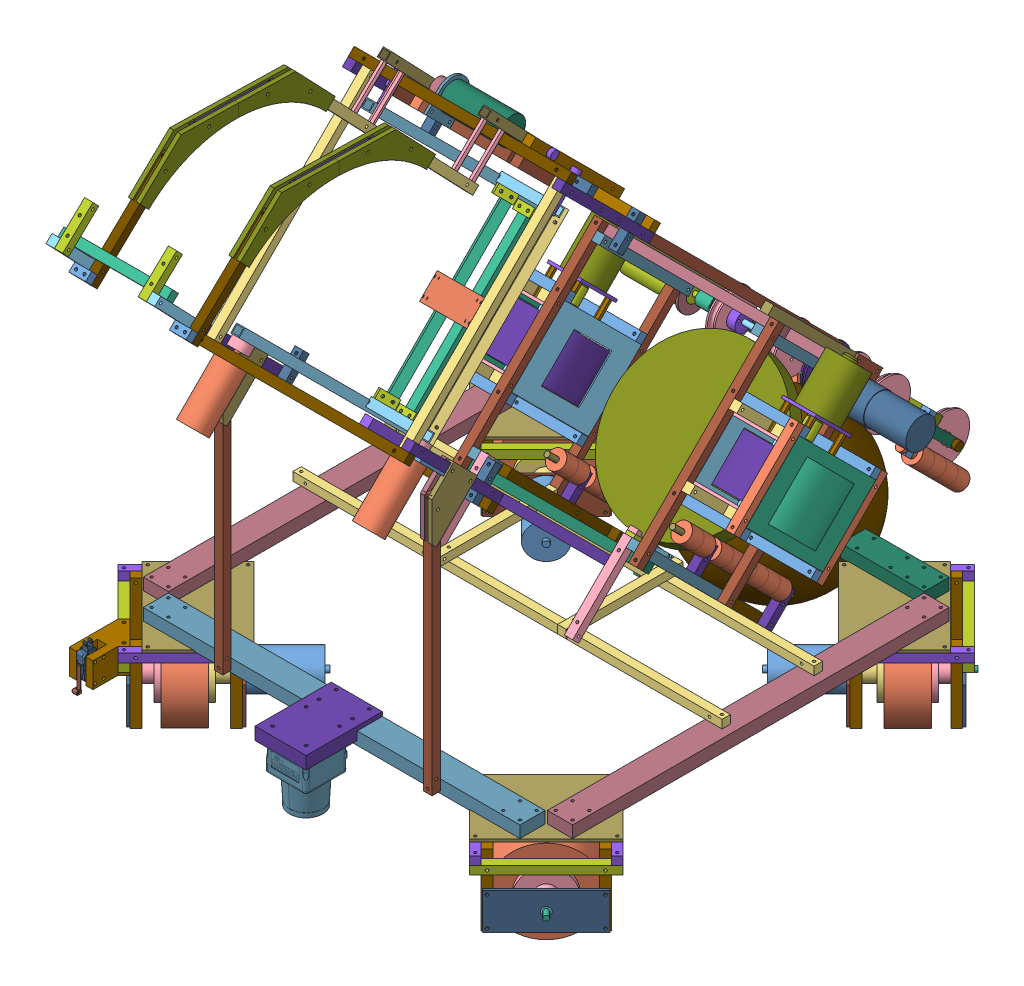
SolidWorks assembly R2, configuration ﾃﾞﾌｫﾙﾄ. Lengths in mm.
Overall size (675.42 1062.97 1046.24).
340 component instances, 123 part files, 65 mates.
Components (placement in the parent):
- Copy of Runner^R2-1: Copy of Runner^R2 [ﾃﾞﾌｫﾙﾄ] at (-280.0303 -23.0504 467.0696) size (603.46 149.94 603.46) (virtual)
  - Copy of Copy of 足回り角^Copy of Runner_R2-1: Copy of Copy of 足回り角^Copy of Runner_R2 [ﾃﾞﾌｫﾙﾄ] at (-236.5804 -569.4039 -424.4309) x (0.322664 -0.429464 -0.843474) z (-0.833839 -0.550655 -0.038606) size (175.41 194.61 181.45) (virtual)
    - Copy of 足回りモータ^Copy of Copy of 足回り角_Copy of Runner_R2-1: Copy of 足回りモータ^Copy of Copy of 足回り角_Copy of Runner_R2 [ﾃﾞﾌｫﾙﾄ] at (-551.1259 26.8519 -574.9243) x (0.279393 -0.550081 -0.786989) z (0.886746 0.462184 -0.008244) size (42 98.4 42) (virtual)
    - Copy of 足回りE^Copy of Copy of 足回り角_Copy of Runner_R2-1: Copy of 足回りE^Copy of Copy of 足回り角_Copy of Runner_R2 [ﾃﾞﾌｫﾙﾄ] at (-524.7579 -22.9499 -530.7534) x (0.201013 -0.588283 -0.783273) z (0.907729 0.412462 -0.07683) size (100 40 100) (virtual)
    - Copy of Part11^Copy of Copy of 足回り角_Copy of Runner_R2-1: Copy of Part11^Copy of Copy of 足回り角_Copy of Runner_R2 [ﾃﾞﾌｫﾙﾄ] at (-688.5751 -7.1777 -584.6401) x (-0.368269 0.695555 -0.616912) z (-0.201013 0.588283 0.783273) size (26.4 56.8 56.8) (virtual)
    - Copy of Copy of Part11^Copy of Copy of 足回り角_Copy of Runner_R2-1: Copy of Copy of Part11^Copy of Copy of 足回り角_Copy of Runner_R2 [ﾃﾞﾌｫﾙﾄ] at (-522.8714 -163.2458 -585.4385) x (0.368269 -0.695555 0.616912) z (0.915702 0.156572 -0.370101) size (26.4 56.8 56.8) (virtual)
    - Part4^Copy of Copy of 足回り角_Copy of Runner_R2-7: Part4^Copy of Copy of 足回り角_Copy of Runner_R2 [ﾃﾞﾌｫﾙﾄ] at (-186.4359 394.8707 -734.6433) x (-0.368269 0.695555 -0.616912) z (0.907729 0.412462 -0.07683) size (2 10 10) (virtual)
    - Part5^Copy of Copy of 足回り角_Copy of Runner_R2-1: Part5^Copy of Copy of 足回り角_Copy of Runner_R2 [ﾃﾞﾌｫﾙﾄ] at (-68.1457 171.4539 -536.4872) x (0.907729 0.412462 -0.07683) z (0.368269 -0.695555 0.616912) size (6 6 35) (virtual)
    - Part6^Copy of Copy of 足回り角_Copy of Runner_R2-12: Part6^Copy of Copy of 足回り角_Copy of Runner_R2 [ﾃﾞﾌｫﾙﾄ] at (-467.3947 -89.0148 -566.7968) x (0.824584 -0.062152 -0.562315) z (-0.429464 -0.715779 -0.550655) size (130 10 10) (virtual)
    - Part6^Copy of Copy of 足回り角_Copy of Runner_R2-16: Part6^Copy of Copy of 足回り角_Copy of Runner_R2 [ﾃﾞﾌｫﾙﾄ] at (-520.2575 -4.441 -653.6633) x (0.824584 -0.062152 -0.562315) z (0.429464 0.715779 0.550655) size (130 10 10) (virtual)
    - Copy of Part6^Copy of Copy of 足回り角_Copy of Runner_R2-7: Copy of Part6^Copy of Copy of 足回り角_Copy of Runner_R2 [ﾃﾞﾌｫﾙﾄ] at (-544.6117 -11.2666 -643.957) x (-0.368269 0.695555 -0.616912) z (0.429464 0.715779 0.550655) size (115 10 10) (virtual)
    - Copy of Part6^Copy of Copy of 足回り角_Copy of Runner_R2-9: Copy of Part6^Copy of Copy of 足回り角_Copy of Runner_R2 [ﾃﾞﾌｫﾙﾄ] at (-643.5618 -3.8083 -576.4793) x (-0.368269 0.695555 -0.616912) z (0.429464 0.715779 0.550655) size (115 10 10) (virtual)
    - Copy of Copy of Part6^Copy of Copy of 足回り角_Copy of Runner_R2-1: Copy of Copy of Part6^Copy of Copy of 足回り角_Copy of Runner_R2 [ﾃﾞﾌｫﾙﾄ] at (-546.4038 -4.8062 -484.4742) x (0.429464 0.715779 0.550655) z (-0.824584 0.062152 0.562315) size (85 10 10) (virtual)
    - Copy of Copy of Part6^Copy of Copy of 足回り角_Copy of Runner_R2-2: Copy of Copy of Part6^Copy of Copy of 足回り角_Copy of Runner_R2 [ﾃﾞﾌｫﾙﾄ] at (-577.7066 54.316 -536.9118) x (0.429464 0.715779 0.550655) z (-0.824584 0.062152 0.562315) size (85 10 10) (virtual)
    - Copy of Copy of Part6^Copy of Copy of 足回り角_Copy of Runner_R2-3: Copy of Copy of Part6^Copy of Copy of 足回り角_Copy of Runner_R2 [ﾃﾞﾌｫﾙﾄ] at (-463.9454 -11.0215 -540.7057) x (0.429464 0.715779 0.550655) z (-0.824584 0.062152 0.562315) size (85 10 10) (virtual)
    - Copy of Copy of Part6^Copy of Copy of 足回り角_Copy of Runner_R2-4: Copy of Copy of Part6^Copy of Copy of 足回り角_Copy of Runner_R2 [ﾃﾞﾌｫﾙﾄ] at (-495.2482 48.1008 -593.1432) x (0.429464 0.715779 0.550655) z (-0.824584 0.062152 0.562315) size (85 10 10) (virtual)
    - Copy of Part7^Copy of Copy of 足回り角_Copy of Runner_R2-1: Copy of Part7^Copy of Copy of 足回り角_Copy of Runner_R2 [ﾃﾞﾌｫﾙﾄ] at (-536.2553 -8.1719 -459.5715) x (0.429464 0.715779 0.550655) z (-0.368269 0.695555 -0.616912) size (43 108 3) (virtual)
    - Part7^Copy of Copy of 足回り角_Copy of Runner_R2-3: Part7^Copy of Copy of 足回り角_Copy of Runner_R2 [ﾃﾞﾌｫﾙﾄ] at (-584.534 59.789 -512.9824) x (0.429464 0.715779 0.550655) z (-0.368269 0.695555 -0.616912) size (43 108 3) (virtual)
    - Part10^Copy of Copy of 足回り角_Copy of Runner_R2-2: Part10^Copy of Copy of 足回り角_Copy of Runner_R2 [ﾃﾞﾌｫﾙﾄ] at (-643.5618 -3.8083 -576.4793) x (0.368269 -0.695555 0.616912) z (-0.429464 -0.715779 -0.550655) size (94.7 130 3) (virtual)
  - Copy of Copy of 足回り角^Copy of Runner_R2-2: Copy of Copy of 足回り角^Copy of Runner_R2 [ﾃﾞﾌｫﾙﾄ] at (937.2593 -569.4039 -236.5804) x (0.843474 -0.429464 0.322664) z (0.038606 -0.550655 -0.833839) size (175.41 194.61 181.45) (virtual)
    - Copy of 足回りモータ^Copy of Copy of 足回り角_Copy of Runner_R2-1: Copy of 足回りモータ^Copy of Copy of 足回り角_Copy of Runner_R2 [ﾃﾞﾌｫﾙﾄ] at (-551.1259 26.8519 -574.9243) x (0.279393 -0.550081 -0.786989) z (0.886746 0.462184 -0.008244) size (42 98.4 42) (virtual)
    - Copy of 足回りE^Copy of Copy of 足回り角_Copy of Runner_R2-1: Copy of 足回りE^Copy of Copy of 足回り角_Copy of Runner_R2 [ﾃﾞﾌｫﾙﾄ] at (-524.7579 -22.9499 -530.7534) x (0.201013 -0.588283 -0.783273) z (0.907729 0.412462 -0.07683) size (100 40 100) (virtual)
    - Copy of Part11^Copy of Copy of 足回り角_Copy of Runner_R2-1: Copy of Part11^Copy of Copy of 足回り角_Copy of Runner_R2 [ﾃﾞﾌｫﾙﾄ] at (-688.5751 -7.1777 -584.6401) x (-0.368269 0.695555 -0.616912) z (-0.201013 0.588283 0.783273) size (26.4 56.8 56.8) (virtual)
    - Copy of Copy of Part11^Copy of Copy of 足回り角_Copy of Runner_R2-1: Copy of Copy of Part11^Copy of Copy of 足回り角_Copy of Runner_R2 [ﾃﾞﾌｫﾙﾄ] at (-522.8714 -163.2458 -585.4385) x (0.368269 -0.695555 0.616912) z (0.915702 0.156572 -0.370101) size (26.4 56.8 56.8) (virtual)
    - Part4^Copy of Copy of 足回り角_Copy of Runner_R2-7: Part4^Copy of Copy of 足回り角_Copy of Runner_R2 [ﾃﾞﾌｫﾙﾄ] at (-186.4359 394.8707 -734.6433) x (-0.368269 0.695555 -0.616912) z (0.907729 0.412462 -0.07683) size (2 10 10) (virtual)
    - Part5^Copy of Copy of 足回り角_Copy of Runner_R2-1: Part5^Copy of Copy of 足回り角_Copy of Runner_R2 [ﾃﾞﾌｫﾙﾄ] at (-68.1457 171.4539 -536.4872) x (0.907729 0.412462 -0.07683) z (0.368269 -0.695555 0.616912) size (6 6 35) (virtual)
    - Part6^Copy of Copy of 足回り角_Copy of Runner_R2-12: Part6^Copy of Copy of 足回り角_Copy of Runner_R2 [ﾃﾞﾌｫﾙﾄ] at (-467.3947 -89.0148 -566.7968) x (0.824584 -0.062152 -0.562315) z (-0.429464 -0.715779 -0.550655) size (130 10 10) (virtual)
    - Part6^Copy of Copy of 足回り角_Copy of Runner_R2-16: Part6^Copy of Copy of 足回り角_Copy of Runner_R2 [ﾃﾞﾌｫﾙﾄ] at (-520.2575 -4.441 -653.6633) x (0.824584 -0.062152 -0.562315) z (0.429464 0.715779 0.550655) size (130 10 10) (virtual)
    - Copy of Part6^Copy of Copy of 足回り角_Copy of Runner_R2-7: Copy of Part6^Copy of Copy of 足回り角_Copy of Runner_R2 [ﾃﾞﾌｫﾙﾄ] at (-544.6117 -11.2666 -643.957) x (-0.368269 0.695555 -0.616912) z (0.429464 0.715779 0.550655) size (115 10 10) (virtual)
    - Copy of Part6^Copy of Copy of 足回り角_Copy of Runner_R2-9: Copy of Part6^Copy of Copy of 足回り角_Copy of Runner_R2 [ﾃﾞﾌｫﾙﾄ] at (-643.5618 -3.8083 -576.4793) x (-0.368269 0.695555 -0.616912) z (0.429464 0.715779 0.550655) size (115 10 10) (virtual)
    - Copy of Copy of Part6^Copy of Copy of 足回り角_Copy of Runner_R2-1: Copy of Copy of Part6^Copy of Copy of 足回り角_Copy of Runner_R2 [ﾃﾞﾌｫﾙﾄ] at (-546.4038 -4.8062 -484.4742) x (0.429464 0.715779 0.550655) z (-0.824584 0.062152 0.562315) size (85 10 10) (virtual)
    - Copy of Copy of Part6^Copy of Copy of 足回り角_Copy of Runner_R2-2: Copy of Copy of Part6^Copy of Copy of 足回り角_Copy of Runner_R2 [ﾃﾞﾌｫﾙﾄ] at (-577.7066 54.316 -536.9118) x (0.429464 0.715779 0.550655) z (-0.824584 0.062152 0.562315) size (85 10 10) (virtual)
    - Copy of Copy of Part6^Copy of Copy of 足回り角_Copy of Runner_R2-3: Copy of Copy of Part6^Copy of Copy of 足回り角_Copy of Runner_R2 [ﾃﾞﾌｫﾙﾄ] at (-463.9454 -11.0215 -540.7057) x (0.429464 0.715779 0.550655) z (-0.824584 0.062152 0.562315) size (85 10 10) (virtual)
    - Copy of Copy of Part6^Copy of Copy of 足回り角_Copy of Runner_R2-4: Copy of Copy of Part6^Copy of Copy of 足回り角_Copy of Runner_R2 [ﾃﾞﾌｫﾙﾄ] at (-495.2482 48.1008 -593.1432) x (0.429464 0.715779 0.550655) z (-0.824584 0.062152 0.562315) size (85 10 10) (virtual)
    - Copy of Part7^Copy of Copy of 足回り角_Copy of Runner_R2-1: Copy of Part7^Copy of Copy of 足回り角_Copy of Runner_R2 [ﾃﾞﾌｫﾙﾄ] at (-536.2553 -8.1719 -459.5715) x (0.429464 0.715779 0.550655) z (-0.368269 0.695555 -0.616912) size (43 108 3) (virtual)
    - Part7^Copy of Copy of 足回り角_Copy of Runner_R2-3: Part7^Copy of Copy of 足回り角_Copy of Runner_R2 [ﾃﾞﾌｫﾙﾄ] at (-584.534 59.789 -512.9824) x (0.429464 0.715779 0.550655) z (-0.368269 0.695555 -0.616912) size (43 108 3) (virtual)
    - Part10^Copy of Copy of 足回り角_Copy of Runner_R2-2: Part10^Copy of Copy of 足回り角_Copy of Runner_R2 [ﾃﾞﾌｫﾙﾄ] at (-643.5618 -3.8083 -576.4793) x (0.368269 -0.695555 0.616912) z (-0.429464 -0.715779 -0.550655) size (94.7 130 3) (virtual)
  - Copy of Copy of 足回り角^Copy of Runner_R2-3: Copy of Copy of 足回り角^Copy of Runner_R2 [ﾃﾞﾌｫﾙﾄ] at (-424.4309 -569.4039 749.4088) x (-0.843474 -0.429464 -0.322664) z (-0.038606 -0.550655 0.833839) size (175.41 194.61 181.45) (virtual)
    - Copy of 足回りモータ^Copy of Copy of 足回り角_Copy of Runner_R2-1: Copy of 足回りモータ^Copy of Copy of 足回り角_Copy of Runner_R2 [ﾃﾞﾌｫﾙﾄ] at (-551.1259 26.8519 -574.9243) x (0.279393 -0.550081 -0.786989) z (0.886746 0.462184 -0.008244) size (42 98.4 42) (virtual)
    - Copy of 足回りE^Copy of Copy of 足回り角_Copy of Runner_R2-1: Copy of 足回りE^Copy of Copy of 足回り角_Copy of Runner_R2 [ﾃﾞﾌｫﾙﾄ] at (-524.7579 -22.9499 -530.7534) x (0.201013 -0.588283 -0.783273) z (0.907729 0.412462 -0.07683) size (100 40 100) (virtual)
    - Copy of Part11^Copy of Copy of 足回り角_Copy of Runner_R2-1: Copy of Part11^Copy of Copy of 足回り角_Copy of Runner_R2 [ﾃﾞﾌｫﾙﾄ] at (-688.5751 -7.1777 -584.6401) x (-0.368269 0.695555 -0.616912) z (-0.201013 0.588283 0.783273) size (26.4 56.8 56.8) (virtual)
    - Copy of Copy of Part11^Copy of Copy of 足回り角_Copy of Runner_R2-1: Copy of Copy of Part11^Copy of Copy of 足回り角_Copy of Runner_R2 [ﾃﾞﾌｫﾙﾄ] at (-522.8714 -163.2458 -585.4385) x (0.368269 -0.695555 0.616912) z (0.915702 0.156572 -0.370101) size (26.4 56.8 56.8) (virtual)
    - Part4^Copy of Copy of 足回り角_Copy of Runner_R2-7: Part4^Copy of Copy of 足回り角_Copy of Runner_R2 [ﾃﾞﾌｫﾙﾄ] at (-186.4359 394.8707 -734.6433) x (-0.368269 0.695555 -0.616912) z (0.907729 0.412462 -0.07683) size (2 10 10) (virtual)
    - Part5^Copy of Copy of 足回り角_Copy of Runner_R2-1: Part5^Copy of Copy of 足回り角_Copy of Runner_R2 [ﾃﾞﾌｫﾙﾄ] at (-68.1457 171.4539 -536.4872) x (0.907729 0.412462 -0.07683) z (0.368269 -0.695555 0.616912) size (6 6 35) (virtual)
    - Part6^Copy of Copy of 足回り角_Copy of Runner_R2-12: Part6^Copy of Copy of 足回り角_Copy of Runner_R2 [ﾃﾞﾌｫﾙﾄ] at (-467.3947 -89.0148 -566.7968) x (0.824584 -0.062152 -0.562315) z (-0.429464 -0.715779 -0.550655) size (130 10 10) (virtual)
    - Part6^Copy of Copy of 足回り角_Copy of Runner_R2-16: Part6^Copy of Copy of 足回り角_Copy of Runner_R2 [ﾃﾞﾌｫﾙﾄ] at (-520.2575 -4.441 -653.6633) x (0.824584 -0.062152 -0.562315) z (0.429464 0.715779 0.550655) size (130 10 10) (virtual)
    - Copy of Part6^Copy of Copy of 足回り角_Copy of Runner_R2-7: Copy of Part6^Copy of Copy of 足回り角_Copy of Runner_R2 [ﾃﾞﾌｫﾙﾄ] at (-544.6117 -11.2666 -643.957) x (-0.368269 0.695555 -0.616912) z (0.429464 0.715779 0.550655) size (115 10 10) (virtual)
    - Copy of Part6^Copy of Copy of 足回り角_Copy of Runner_R2-9: Copy of Part6^Copy of Copy of 足回り角_Copy of Runner_R2 [ﾃﾞﾌｫﾙﾄ] at (-643.5618 -3.8083 -576.4793) x (-0.368269 0.695555 -0.616912) z (0.429464 0.715779 0.550655) size (115 10 10) (virtual)
    - Copy of Copy of Part6^Copy of Copy of 足回り角_Copy of Runner_R2-1: Copy of Copy of Part6^Copy of Copy of 足回り角_Copy of Runner_R2 [ﾃﾞﾌｫﾙﾄ] at (-546.4038 -4.8062 -484.4742) x (0.429464 0.715779 0.550655) z (-0.824584 0.062152 0.562315) size (85 10 10) (virtual)
    - Copy of Copy of Part6^Copy of Copy of 足回り角_Copy of Runner_R2-2: Copy of Copy of Part6^Copy of Copy of 足回り角_Copy of Runner_R2 [ﾃﾞﾌｫﾙﾄ] at (-577.7066 54.316 -536.9118) x (0.429464 0.715779 0.550655) z (-0.824584 0.062152 0.562315) size (85 10 10) (virtual)
    - Copy of Copy of Part6^Copy of Copy of 足回り角_Copy of Runner_R2-3: Copy of Copy of Part6^Copy of Copy of 足回り角_Copy of Runner_R2 [ﾃﾞﾌｫﾙﾄ] at (-463.9454 -11.0215 -540.7057) x (0.429464 0.715779 0.550655) z (-0.824584 0.062152 0.562315) size (85 10 10) (virtual)
    - Copy of Copy of Part6^Copy of Copy of 足回り角_Copy of Runner_R2-4: Copy of Copy of Part6^Copy of Copy of 足回り角_Copy of Runner_R2 [ﾃﾞﾌｫﾙﾄ] at (-495.2482 48.1008 -593.1432) x (0.429464 0.715779 0.550655) z (-0.824584 0.062152 0.562315) size (85 10 10) (virtual)
    - Copy of Part7^Copy of Copy of 足回り角_Copy of Runner_R2-1: Copy of Part7^Copy of Copy of 足回り角_Copy of Runner_R2 [ﾃﾞﾌｫﾙﾄ] at (-536.2553 -8.1719 -459.5715) x (0.429464 0.715779 0.550655) z (-0.368269 0.695555 -0.616912) size (43 108 3) (virtual)
    - Part7^Copy of Copy of 足回り角_Copy of Runner_R2-3: Part7^Copy of Copy of 足回り角_Copy of Runner_R2 [ﾃﾞﾌｫﾙﾄ] at (-584.534 59.789 -512.9824) x (0.429464 0.715779 0.550655) z (-0.368269 0.695555 -0.616912) size (43 108 3) (virtual)
    - Part10^Copy of Copy of 足回り角_Copy of Runner_R2-2: Part10^Copy of Copy of 足回り角_Copy of Runner_R2 [ﾃﾞﾌｫﾙﾄ] at (-643.5618 -3.8083 -576.4793) x (0.368269 -0.695555 0.616912) z (-0.429464 -0.715779 -0.550655) size (94.7 130 3) (virtual)
  - Copy of Copy of 足回り角^Copy of Runner_R2-4: Copy of Copy of 足回り角^Copy of Runner_R2 [ﾃﾞﾌｫﾙﾄ] at (749.4088 -569.4039 937.2593) x (-0.322664 -0.429464 0.843474) z (0.833839 -0.550655 0.038606) size (175.41 194.61 181.45) (virtual)
    - Copy of 足回りモータ^Copy of Copy of 足回り角_Copy of Runner_R2-1: Copy of 足回りモータ^Copy of Copy of 足回り角_Copy of Runner_R2 [ﾃﾞﾌｫﾙﾄ] at (-551.1259 26.8519 -574.9243) x (0.279393 -0.550081 -0.786989) z (0.886746 0.462184 -0.008244) size (42 98.4 42) (virtual)
    - Copy of 足回りE^Copy of Copy of 足回り角_Copy of Runner_R2-1: Copy of 足回りE^Copy of Copy of 足回り角_Copy of Runner_R2 [ﾃﾞﾌｫﾙﾄ] at (-524.7579 -22.9499 -530.7534) x (0.201013 -0.588283 -0.783273) z (0.907729 0.412462 -0.07683) size (100 40 100) (virtual)
    - Copy of Part11^Copy of Copy of 足回り角_Copy of Runner_R2-1: Copy of Part11^Copy of Copy of 足回り角_Copy of Runner_R2 [ﾃﾞﾌｫﾙﾄ] at (-688.5751 -7.1777 -584.6401) x (-0.368269 0.695555 -0.616912) z (-0.201013 0.588283 0.783273) size (26.4 56.8 56.8) (virtual)
    - Copy of Copy of Part11^Copy of Copy of 足回り角_Copy of Runner_R2-1: Copy of Copy of Part11^Copy of Copy of 足回り角_Copy of Runner_R2 [ﾃﾞﾌｫﾙﾄ] at (-522.8714 -163.2458 -585.4385) x (0.368269 -0.695555 0.616912) z (0.915702 0.156572 -0.370101) size (26.4 56.8 56.8) (virtual)
    - Part4^Copy of Copy of 足回り角_Copy of Runner_R2-7: Part4^Copy of Copy of 足回り角_Copy of Runner_R2 [ﾃﾞﾌｫﾙﾄ] at (-186.4359 394.8707 -734.6433) x (-0.368269 0.695555 -0.616912) z (0.907729 0.412462 -0.07683) size (2 10 10) (virtual)
    - Part5^Copy of Copy of 足回り角_Copy of Runner_R2-1: Part5^Copy of Copy of 足回り角_Copy of Runner_R2 [ﾃﾞﾌｫﾙﾄ] at (-68.1457 171.4539 -536.4872) x (0.907729 0.412462 -0.07683) z (0.368269 -0.695555 0.616912) size (6 6 35) (virtual)
    - Part6^Copy of Copy of 足回り角_Copy of Runner_R2-12: Part6^Copy of Copy of 足回り角_Copy of Runner_R2 [ﾃﾞﾌｫﾙﾄ] at (-467.3947 -89.0148 -566.7968) x (0.824584 -0.062152 -0.562315) z (-0.429464 -0.715779 -0.550655) size (130 10 10) (virtual)
    - Part6^Copy of Copy of 足回り角_Copy of Runner_R2-16: Part6^Copy of Copy of 足回り角_Copy of Runner_R2 [ﾃﾞﾌｫﾙﾄ] at (-520.2575 -4.441 -653.6633) x (0.824584 -0.062152 -0.562315) z (0.429464 0.715779 0.550655) size (130 10 10) (virtual)
    - Copy of Part6^Copy of Copy of 足回り角_Copy of Runner_R2-7: Copy of Part6^Copy of Copy of 足回り角_Copy of Runner_R2 [ﾃﾞﾌｫﾙﾄ] at (-544.6117 -11.2666 -643.957) x (-0.368269 0.695555 -0.616912) z (0.429464 0.715779 0.550655) size (115 10 10) (virtual)
    - Copy of Part6^Copy of Copy of 足回り角_Copy of Runner_R2-9: Copy of Part6^Copy of Copy of 足回り角_Copy of Runner_R2 [ﾃﾞﾌｫﾙﾄ] at (-643.5618 -3.8083 -576.4793) x (-0.368269 0.695555 -0.616912) z (0.429464 0.715779 0.550655) size (115 10 10) (virtual)
    - Copy of Copy of Part6^Copy of Copy of 足回り角_Copy of Runner_R2-1: Copy of Copy of Part6^Copy of Copy of 足回り角_Copy of Runner_R2 [ﾃﾞﾌｫﾙﾄ] at (-546.4038 -4.8062 -484.4742) x (0.429464 0.715779 0.550655) z (-0.824584 0.062152 0.562315) size (85 10 10) (virtual)
    - Copy of Copy of Part6^Copy of Copy of 足回り角_Copy of Runner_R2-2: Copy of Copy of Part6^Copy of Copy of 足回り角_Copy of Runner_R2 [ﾃﾞﾌｫﾙﾄ] at (-577.7066 54.316 -536.9118) x (0.429464 0.715779 0.550655) z (-0.824584 0.062152 0.562315) size (85 10 10) (virtual)
    - Copy of Copy of Part6^Copy of Copy of 足回り角_Copy of Runner_R2-3: Copy of Copy of Part6^Copy of Copy of 足回り角_Copy of Runner_R2 [ﾃﾞﾌｫﾙﾄ] at (-463.9454 -11.0215 -540.7057) x (0.429464 0.715779 0.550655) z (-0.824584 0.062152 0.562315) size (85 10 10) (virtual)
    - Copy of Copy of Part6^Copy of Copy of 足回り角_Copy of Runner_R2-4: Copy of Copy of Part6^Copy of Copy of 足回り角_Copy of Runner_R2 [ﾃﾞﾌｫﾙﾄ] at (-495.2482 48.1008 -593.1432) x (0.429464 0.715779 0.550655) z (-0.824584 0.062152 0.562315) size (85 10 10) (virtual)
    - Copy of Part7^Copy of Copy of 足回り角_Copy of Runner_R2-1: Copy of Part7^Copy of Copy of 足回り角_Copy of Runner_R2 [ﾃﾞﾌｫﾙﾄ] at (-536.2553 -8.1719 -459.5715) x (0.429464 0.715779 0.550655) z (-0.368269 0.695555 -0.616912) size (43 108 3) (virtual)
    - Part7^Copy of Copy of 足回り角_Copy of Runner_R2-3: Part7^Copy of Copy of 足回り角_Copy of Runner_R2 [ﾃﾞﾌｫﾙﾄ] at (-584.534 59.789 -512.9824) x (0.429464 0.715779 0.550655) z (-0.368269 0.695555 -0.616912) size (43 108 3) (virtual)
    - Part10^Copy of Copy of 足回り角_Copy of Runner_R2-2: Part10^Copy of Copy of 足回り角_Copy of Runner_R2 [ﾃﾞﾌｫﾙﾄ] at (-643.5618 -3.8083 -576.4793) x (0.368269 -0.695555 0.616912) z (-0.429464 -0.715779 -0.550655) size (94.7 130 3) (virtual)
  - Part9^Copy of Runner_R2-1: Part9^Copy of Runner_R2 [ﾃﾞﾌｫﾙﾄ] at (521.6964 29.1498 330.8565) x (0 0 -1) z (0 1 0) size (450 30 15) (virtual)
  - Copy of Part9^Copy of Runner_R2-1: Copy of Part9^Copy of Runner_R2 [ﾃﾞﾌｫﾙﾄ] at (330.3437 44.1498 521.6964) x (-1 0 0) z (0 -1 0) size (450 30 15) (virtual)
  - Part9^Copy of Runner_R2-3: Part9^Copy of Runner_R2 [ﾃﾞﾌｫﾙﾄ] at (-8.868 29.1498 181.972) x (0 0 1) z (0 1 0) size (450 30 15) (virtual)
  - Copy (2) of Part9^Copy of Runner_R2-1: Copy (2) of Part9^Copy of Runner_R2 [ﾃﾞﾌｫﾙﾄ] at (-19.1435 29.1498 -8.868) x (-1 0 0) z (0 1 0) size (100 30 15) (virtual)
  - Copy (2) of Part9^Copy of Runner_R2-2: Copy (2) of Part9^Copy of Runner_R2 [ﾃﾞﾌｫﾙﾄ] at (531.972 29.1498 38.868) x (1 0 0) z (0 1 0) size (100 30 15) (virtual)
- Copy of Shooter^R2-1: Copy of Shooter^R2 [ﾃﾞﾌｫﾙﾄ] at (-133.6019 -3.3981 619.3345) x (1 0 0) z (0 0.707107 0.707107) size (512.8 347.34 409.41) (virtual, flexible)
  - Copy of Roller^Copy of Shooter_R2-1: Copy of Roller^Copy of Shooter_R2 [ﾃﾞﾌｫﾙﾄ] at (-59.3841 78.5441 92.0532) x (0.999685 0 0.025079) z (-0.025079 0 0.999685) size (101.44 180.8 151.71) (virtual)
    - Copy of Copy of motor^Copy of Roller_Copy of Shooter_R2-1: Copy of Copy of motor^Copy of Roller_Copy of Shooter_R2 [ﾃﾞﾌｫﾙﾄ] at (28.9472 162.9559 -17.7848) x (0.025079 0 0.999685) z (0 -1 0) size (45 45 69.7) (virtual)
    - Part5^Copy of Roller_Copy of Shooter_R2-1: Part5^Copy of Roller_Copy of Shooter_R2 [ﾃﾞﾌｫﾙﾄ] at (28.9472 14.4559 -17.7848) x (0.999895 0 0.0145) z (-0.0145 0 0.999895) size (100 54 100) (virtual)
    - Part6^Copy of Roller_Copy of Shooter_R2-1: Part6^Copy of Roller_Copy of Shooter_R2 [ﾃﾞﾌｫﾙﾄ] at (28.9472 29.4559 -17.7848) x (-0.999895 0 -0.0145) z (-0.0145 0 0.999895) size (28 15 28) (virtual)
    - Copy of Copy (2) of Copy of Copy (2) of 角材１^Copy of Roller_Copy of Shooter_R2-1: Copy of Copy (2) of Copy of Copy (2) of 角材１^Copy of Roller_Copy of Shooter_R2 [ﾃﾞﾌｫﾙﾄ] at (-9.6609 -13.5441 38.2011) x (0.999685 0 -0.025079) z (0.025079 0 0.999685) size (80 10 10) (virtual)
    - Copy of Copy (2) of Copy of Copy (2) of 角材１^Copy of Roller_Copy of Shooter_R2-2: Copy of Copy (2) of Copy of Copy (2) of 角材１^Copy of Roller_Copy of Shooter_R2 [ﾃﾞﾌｫﾙﾄ] at (-12.6704 -13.5441 -81.7612) x (0.999685 0 -0.025079) z (0.025079 0 0.999685) size (80 10 10) (virtual)
    - Copy of Copy of Copy (2) of Copy of Copy (2) of 角材１^Copy of Roller_Copy of Shooter_R2-2: Copy of Copy of Copy (2) of Copy of Copy (2) of 角材１^Copy of Roller_Copy of Shooter_R2 [ﾃﾞﾌｫﾙﾄ] at (-9.4101 96.4559 48.1979) x (0 -1 0) z (0.025079 0 0.999685) size (110 10 10) (virtual)
    - Copy of Copy of Copy (2) of Copy of Copy (2) of 角材１^Copy of Roller_Copy of Shooter_R2-4: Copy of Copy of Copy (2) of Copy of Copy (2) of 角材１^Copy of Roller_Copy of Shooter_R2 [ﾃﾞﾌｫﾙﾄ] at (-12.9212 96.4559 -91.7581) x (0 -1 0) z (0.025079 0 0.999685) size (110 10 10) (virtual)
    - Copy (2) of Copy of Copy (2) of Copy of Copy (2) of 角材１^Copy of Roller_Copy of Shooter_R2-1: Copy (2) of Copy of Copy (2) of Copy of Copy (2) of 角材１^Copy of Roller_Copy of Shooter_R2 [ﾃﾞﾌｫﾙﾄ] at (57.0568 -3.5441 -93.5136) x (0.025079 0 0.999685) z (-0.999685 0 0.025079) size (150 10 10) (virtual)
    - Copy (2) of Copy of Copy (2) of Copy of Copy (2) of 角材１^Copy of Roller_Copy of Shooter_R2-2: Copy (2) of Copy of Copy (2) of Copy of Copy (2) of 角材１^Copy of Roller_Copy of Shooter_R2 [ﾃﾞﾌｫﾙﾄ] at (7.0725 -3.5441 -92.2596) x (0.025079 0 0.999685) z (-0.999685 0 0.025079) size (150 10 10) (virtual)
    - Copy (2) of Copy of Copy (2) of Copy of Copy (2) of 角材１^Copy of Roller_Copy of Shooter_R2-3: Copy (2) of Copy of Copy (2) of Copy of Copy (2) of 角材１^Copy of Roller_Copy of Shooter_R2 [ﾃﾞﾌｫﾙﾄ] at (7.0725 76.4559 -92.2596) x (0.025079 0 0.999685) z (-0.999685 0 0.025079) size (150 10 10) (virtual)
    - Copy (2) of Copy of Copy (2) of Copy of Copy (2) of 角材１^Copy of Roller_Copy of Shooter_R2-4: Copy (2) of Copy of Copy (2) of Copy of Copy (2) of 角材１^Copy of Roller_Copy of Shooter_R2 [ﾃﾞﾌｫﾙﾄ] at (57.0568 76.4559 -93.5136) x (0.025079 0 0.999685) z (-0.999685 0 0.025079) size (150 10 10) (virtual)
    - Copy of Copy (2) of Copy of Copy (2) of 角材１^Copy of Roller_Copy of Shooter_R2-5: Copy of Copy (2) of Copy of Copy (2) of 角材１^Copy of Roller_Copy of Shooter_R2 [ﾃﾞﾌｫﾙﾄ] at (-12.6704 86.4559 -81.7612) x (0.999685 0 -0.025079) z (0.025079 0 0.999685) size (80 10 10) (virtual)
    - Copy of Copy (2) of Copy of Copy (2) of 角材１^Copy of Roller_Copy of Shooter_R2-6: Copy of Copy (2) of Copy of Copy (2) of 角材１^Copy of Roller_Copy of Shooter_R2 [ﾃﾞﾌｫﾙﾄ] at (-9.6609 86.4559 38.2011) x (0.999685 0 -0.025079) z (0.025079 0 0.999685) size (80 10 10) (virtual)
    - Part8^Copy of Roller_Copy of Shooter_R2-1: Part8^Copy of Roller_Copy of Shooter_R2 [ﾃﾞﾌｫﾙﾄ] at (-2.6735 6.4559 -82.012) x (0.025079 0 0.999685) z (0 1 0) size (130 60 3) (virtual)
    - Part9^Copy of Roller_Copy of Shooter_R2-1: Part9^Copy of Roller_Copy of Shooter_R2 [ﾃﾞﾌｫﾙﾄ] at (13.5757 9.4559 -32.4039) x (0.025079 0 0.999685) z (0 1 0) size (30 30 7) (virtual)
    - Part8^Copy of Roller_Copy of Shooter_R2-2: Part8^Copy of Roller_Copy of Shooter_R2 [ﾃﾞﾌｫﾙﾄ] at (57.3076 76.4559 -83.5168) x (0.025079 0 0.999685) z (0 -1 0) size (130 60 3) (virtual)
    - Part9^Copy of Roller_Copy of Shooter_R2-2: Part9^Copy of Roller_Copy of Shooter_R2 [ﾃﾞﾌｫﾙﾄ] at (43.5663 73.4559 -33.1563) x (0.025079 0 0.999685) z (0 -1 0) size (30 30 7) (virtual)
    - Part6^Copy of Roller_Copy of Shooter_R2-2: Part6^Copy of Roller_Copy of Shooter_R2 [ﾃﾞﾌｫﾙﾄ] at (28.9472 37.4559 -17.7848) x (0.999895 0 0.0145) z (-0.0145 0 0.999895) size (28 15 28) (virtual)
    - Part11^Copy of Roller_Copy of Shooter_R2-1: Part11^Copy of Roller_Copy of Shooter_R2 [ﾃﾞﾌｫﾙﾄ] at (28.9472 -2.4441 -17.7848) x (0 1 0) z (-0.999993 0 0.003776) size (100 6 6) (virtual)
    - Part12^Copy of Roller_Copy of Shooter_R2-1: Part12^Copy of Roller_Copy of Shooter_R2 [ﾃﾞﾌｫﾙﾄ] at (28.9472 87.0559 -17.7848) x (0.99763 0 -0.068811) z (0 1 0) size (16 16 18) (virtual)
    - Part13^Copy of Roller_Copy of Shooter_R2-1: Part13^Copy of Roller_Copy of Shooter_R2 [ﾃﾞﾌｫﾙﾄ] at (28.9472 109.4559 -17.7848) x (-0.999685 0 0.025079) z (0 -1 0) size (40 60 3) (virtual)
    - Part14^Copy of Roller_Copy of Shooter_R2-1: Part14^Copy of Roller_Copy of Shooter_R2 [ﾃﾞﾌｫﾙﾄ] at (14.5789 76.4559 7.5835) x (-0.003776 0 -0.999993) z (0 1 0) size (6.34 5.64 30) (virtual)
    - Part14^Copy of Roller_Copy of Shooter_R2-2: Part14^Copy of Roller_Copy of Shooter_R2 [ﾃﾞﾌｫﾙﾄ] at (43.3155 76.4559 -43.1531) x (-0.003776 0 -0.999993) z (0 1 0) size (6.34 5.64 30) (virtual)
    - Part14^Copy of Roller_Copy of Shooter_R2-3: Part14^Copy of Roller_Copy of Shooter_R2 [ﾃﾞﾌｫﾙﾄ] at (44.5695 76.4559 6.8311) x (-0.003776 0 -0.999993) z (0 1 0) size (6.34 5.64 30) (virtual)
    - Part14^Copy of Roller_Copy of Shooter_R2-4: Part14^Copy of Roller_Copy of Shooter_R2 [ﾃﾞﾌｫﾙﾄ] at (13.3249 76.4559 -42.4008) x (-0.003776 0 -0.999993) z (0 1 0) size (6.34 5.64 30) (virtual)
    - Part15^Copy of Roller_Copy of Shooter_R2-1: Part15^Copy of Roller_Copy of Shooter_R2 [ﾃﾞﾌｫﾙﾄ] at (28.9472 14.4559 -17.7848) x (0.00379 0 0.999993) z (0 -1 0) size (13 13 5) (virtual)
    - Part15^Copy of Roller_Copy of Shooter_R2-2: Part15^Copy of Roller_Copy of Shooter_R2 [ﾃﾞﾌｫﾙﾄ] at (28.9472 73.4559 -17.7848) x (0.00379 0 0.999993) z (0 -1 0) size (13 13 5) (virtual)
  - Copy of Roller^Copy of Shooter_R2-2: Copy of Roller^Copy of Shooter_R2 [ﾃﾞﾌｫﾙﾄ] at (279.3841 78.5441 57.9468) x (-0.999685 0 -0.025079) z (0.025079 0 -0.999685) size (101.44 180.8 151.71) (virtual)
    - Copy of Copy of motor^Copy of Roller_Copy of Shooter_R2-1: Copy of Copy of motor^Copy of Roller_Copy of Shooter_R2 [ﾃﾞﾌｫﾙﾄ] at (28.9472 162.9559 -17.7848) x (0.025079 0 0.999685) z (0 -1 0) size (45 45 69.7) (virtual)
    - Part5^Copy of Roller_Copy of Shooter_R2-1: Part5^Copy of Roller_Copy of Shooter_R2 [ﾃﾞﾌｫﾙﾄ] at (28.9472 14.4559 -17.7848) x (0.999895 0 0.0145) z (-0.0145 0 0.999895) size (100 54 100) (virtual)
    - Part6^Copy of Roller_Copy of Shooter_R2-1: Part6^Copy of Roller_Copy of Shooter_R2 [ﾃﾞﾌｫﾙﾄ] at (28.9472 29.4559 -17.7848) x (-0.999895 0 -0.0145) z (-0.0145 0 0.999895) size (28 15 28) (virtual)
    - Copy of Copy (2) of Copy of Copy (2) of 角材１^Copy of Roller_Copy of Shooter_R2-1: Copy of Copy (2) of Copy of Copy (2) of 角材１^Copy of Roller_Copy of Shooter_R2 [ﾃﾞﾌｫﾙﾄ] at (-9.6609 -13.5441 38.2011) x (0.999685 0 -0.025079) z (0.025079 0 0.999685) size (80 10 10) (virtual)
    - Copy of Copy (2) of Copy of Copy (2) of 角材１^Copy of Roller_Copy of Shooter_R2-2: Copy of Copy (2) of Copy of Copy (2) of 角材１^Copy of Roller_Copy of Shooter_R2 [ﾃﾞﾌｫﾙﾄ] at (-12.6704 -13.5441 -81.7612) x (0.999685 0 -0.025079) z (0.025079 0 0.999685) size (80 10 10) (virtual)
    - Copy of Copy of Copy (2) of Copy of Copy (2) of 角材１^Copy of Roller_Copy of Shooter_R2-2: Copy of Copy of Copy (2) of Copy of Copy (2) of 角材１^Copy of Roller_Copy of Shooter_R2 [ﾃﾞﾌｫﾙﾄ] at (-9.4101 96.4559 48.1979) x (0 -1 0) z (0.025079 0 0.999685) size (110 10 10) (virtual)
    - Copy of Copy of Copy (2) of Copy of Copy (2) of 角材１^Copy of Roller_Copy of Shooter_R2-4: Copy of Copy of Copy (2) of Copy of Copy (2) of 角材１^Copy of Roller_Copy of Shooter_R2 [ﾃﾞﾌｫﾙﾄ] at (-12.9212 96.4559 -91.7581) x (0 -1 0) z (0.025079 0 0.999685) size (110 10 10) (virtual)
    - Copy (2) of Copy of Copy (2) of Copy of Copy (2) of 角材１^Copy of Roller_Copy of Shooter_R2-1: Copy (2) of Copy of Copy (2) of Copy of Copy (2) of 角材１^Copy of Roller_Copy of Shooter_R2 [ﾃﾞﾌｫﾙﾄ] at (57.0568 -3.5441 -93.5136) x (0.025079 0 0.999685) z (-0.999685 0 0.025079) size (150 10 10) (virtual)
    - Copy (2) of Copy of Copy (2) of Copy of Copy (2) of 角材１^Copy of Roller_Copy of Shooter_R2-2: Copy (2) of Copy of Copy (2) of Copy of Copy (2) of 角材１^Copy of Roller_Copy of Shooter_R2 [ﾃﾞﾌｫﾙﾄ] at (7.0725 -3.5441 -92.2596) x (0.025079 0 0.999685) z (-0.999685 0 0.025079) size (150 10 10) (virtual)
    - Copy (2) of Copy of Copy (2) of Copy of Copy (2) of 角材１^Copy of Roller_Copy of Shooter_R2-3: Copy (2) of Copy of Copy (2) of Copy of Copy (2) of 角材１^Copy of Roller_Copy of Shooter_R2 [ﾃﾞﾌｫﾙﾄ] at (7.0725 76.4559 -92.2596) x (0.025079 0 0.999685) z (-0.999685 0 0.025079) size (150 10 10) (virtual)
    - Copy (2) of Copy of Copy (2) of Copy of Copy (2) of 角材１^Copy of Roller_Copy of Shooter_R2-4: Copy (2) of Copy of Copy (2) of Copy of Copy (2) of 角材１^Copy of Roller_Copy of Shooter_R2 [ﾃﾞﾌｫﾙﾄ] at (57.0568 76.4559 -93.5136) x (0.025079 0 0.999685) z (-0.999685 0 0.025079) size (150 10 10) (virtual)
    - Copy of Copy (2) of Copy of Copy (2) of 角材１^Copy of Roller_Copy of Shooter_R2-5: Copy of Copy (2) of Copy of Copy (2) of 角材１^Copy of Roller_Copy of Shooter_R2 [ﾃﾞﾌｫﾙﾄ] at (-12.6704 86.4559 -81.7612) x (0.999685 0 -0.025079) z (0.025079 0 0.999685) size (80 10 10) (virtual)
    - Copy of Copy (2) of Copy of Copy (2) of 角材１^Copy of Roller_Copy of Shooter_R2-6: Copy of Copy (2) of Copy of Copy (2) of 角材１^Copy of Roller_Copy of Shooter_R2 [ﾃﾞﾌｫﾙﾄ] at (-9.6609 86.4559 38.2011) x (0.999685 0 -0.025079) z (0.025079 0 0.999685) size (80 10 10) (virtual)
    - Part8^Copy of Roller_Copy of Shooter_R2-1: Part8^Copy of Roller_Copy of Shooter_R2 [ﾃﾞﾌｫﾙﾄ] at (-2.6735 6.4559 -82.012) x (0.025079 0 0.999685) z (0 1 0) size (130 60 3) (virtual)
    - Part9^Copy of Roller_Copy of Shooter_R2-1: Part9^Copy of Roller_Copy of Shooter_R2 [ﾃﾞﾌｫﾙﾄ] at (13.5757 9.4559 -32.4039) x (0.025079 0 0.999685) z (0 1 0) size (30 30 7) (virtual)
    - Part8^Copy of Roller_Copy of Shooter_R2-2: Part8^Copy of Roller_Copy of Shooter_R2 [ﾃﾞﾌｫﾙﾄ] at (57.3076 76.4559 -83.5168) x (0.025079 0 0.999685) z (0 -1 0) size (130 60 3) (virtual)
    - Part9^Copy of Roller_Copy of Shooter_R2-2: Part9^Copy of Roller_Copy of Shooter_R2 [ﾃﾞﾌｫﾙﾄ] at (43.5663 73.4559 -33.1563) x (0.025079 0 0.999685) z (0 -1 0) size (30 30 7) (virtual)
    - Part6^Copy of Roller_Copy of Shooter_R2-2: Part6^Copy of Roller_Copy of Shooter_R2 [ﾃﾞﾌｫﾙﾄ] at (28.9472 37.4559 -17.7848) x (0.999895 0 0.0145) z (-0.0145 0 0.999895) size (28 15 28) (virtual)
    - Part11^Copy of Roller_Copy of Shooter_R2-1: Part11^Copy of Roller_Copy of Shooter_R2 [ﾃﾞﾌｫﾙﾄ] at (28.9472 -2.4441 -17.7848) x (0 1 0) z (-0.999993 0 0.003776) size (100 6 6) (virtual)
    - Part12^Copy of Roller_Copy of Shooter_R2-1: Part12^Copy of Roller_Copy of Shooter_R2 [ﾃﾞﾌｫﾙﾄ] at (28.9472 87.0559 -17.7848) x (0.99763 0 -0.068811) z (0 1 0) size (16 16 18) (virtual)
    - Part13^Copy of Roller_Copy of Shooter_R2-1: Part13^Copy of Roller_Copy of Shooter_R2 [ﾃﾞﾌｫﾙﾄ] at (28.9472 109.4559 -17.7848) x (-0.999685 0 0.025079) z (0 -1 0) size (40 60 3) (virtual)
    - Part14^Copy of Roller_Copy of Shooter_R2-1: Part14^Copy of Roller_Copy of Shooter_R2 [ﾃﾞﾌｫﾙﾄ] at (14.5789 76.4559 7.5835) x (-0.003776 0 -0.999993) z (0 1 0) size (6.34 5.64 30) (virtual)
    - Part14^Copy of Roller_Copy of Shooter_R2-2: Part14^Copy of Roller_Copy of Shooter_R2 [ﾃﾞﾌｫﾙﾄ] at (43.3155 76.4559 -43.1531) x (-0.003776 0 -0.999993) z (0 1 0) size (6.34 5.64 30) (virtual)
    - Part14^Copy of Roller_Copy of Shooter_R2-3: Part14^Copy of Roller_Copy of Shooter_R2 [ﾃﾞﾌｫﾙﾄ] at (44.5695 76.4559 6.8311) x (-0.003776 0 -0.999993) z (0 1 0) size (6.34 5.64 30) (virtual)
    - Part14^Copy of Roller_Copy of Shooter_R2-4: Part14^Copy of Roller_Copy of Shooter_R2 [ﾃﾞﾌｫﾙﾄ] at (13.3249 76.4559 -42.4008) x (-0.003776 0 -0.999993) z (0 1 0) size (6.34 5.64 30) (virtual)
    - Part15^Copy of Roller_Copy of Shooter_R2-1: Part15^Copy of Roller_Copy of Shooter_R2 [ﾃﾞﾌｫﾙﾄ] at (28.9472 14.4559 -17.7848) x (0.00379 0 0.999993) z (0 -1 0) size (13 13 5) (virtual)
    - Part15^Copy of Roller_Copy of Shooter_R2-2: Part15^Copy of Roller_Copy of Shooter_R2 [ﾃﾞﾌｫﾙﾄ] at (28.9472 73.4559 -17.7848) x (0.00379 0 0.999993) z (0 -1 0) size (13 13 5) (virtual)
  - Copy of Copy of Copy of Copy of Copy of Copy (2) of Copy of Copy (2) of 角材１^Copy of Shooter_R2-1: Copy of Copy of Copy of Copy of Copy of Copy (2) of Copy of Copy (2) of 角材１^Copy of Shooter_R2 [ﾃﾞﾌｫﾙﾄ] at (0 240 140) x (0 -1 0) z (0 0 1) size (240 10 10) (virtual)
  - Part17^Copy of Shooter_R2-1: Part17^Copy of Shooter_R2 [ﾃﾞﾌｫﾙﾄ] at (185 45 -115) x (0.901476 -0.432829 0) z (0 0 1) size (6 6 200) (virtual)
  - Copy of Copy of Copy of Copy of Copy of Copy (2) of Copy of Copy (2) of 角材１^Copy of Shooter_R2-2: Copy of Copy of Copy of Copy of Copy of Copy (2) of Copy of Copy (2) of 角材１^Copy of Shooter_R2 [ﾃﾞﾌｫﾙﾄ] at (0 240 0) x (0 -1 0) z (0 0 1) size (240 10 10) (virtual)
  - Copy of Copy of Copy of Copy of Copy (2) of Copy of Copy (2) of 角材１^Copy of Shooter_R2-2: Copy of Copy of Copy of Copy of Copy (2) of Copy of Copy (2) of 角材１^Copy of Shooter_R2 [ﾃﾞﾌｫﾙﾄ] at (0 230 10) size (220 10 10) (virtual)
  - Copy of Copy of Copy of Copy of Copy (2) of Copy of Copy (2) of 角材１^Copy of Shooter_R2-5: Copy of Copy of Copy of Copy of Copy (2) of Copy of Copy (2) of 角材１^Copy of Shooter_R2 [ﾃﾞﾌｫﾙﾄ] at (0 230 130) size (220 10 10) (virtual)
  - Copy of Copy of Copy (2) of Copy of Copy (2) of Copy of Copy (2) of 角材１^Copy of Shooter_R2-1: Copy of Copy of Copy (2) of Copy of Copy (2) of Copy of Copy (2) of 角材１^Copy of Shooter_R2 [ﾃﾞﾌｫﾙﾄ] at (20 220 0) x (0 0 1) z (-1 0 0) size (150 10 10) (virtual)
  - Copy of Copy of Copy (2) of Copy of Copy (2) of Copy of Copy (2) of 角材１^Copy of Shooter_R2-2: Copy of Copy of Copy (2) of Copy of Copy (2) of Copy of Copy (2) of 角材１^Copy of Shooter_R2 [ﾃﾞﾌｫﾙﾄ] at (210 220 0) x (0 0 1) z (-1 0 0) size (150 10 10) (virtual)
  - Copy of Copy of Copy of Copy of Copy of Copy (2) of Copy of Copy (2) of 角材１^Copy of Shooter_R2-3: Copy of Copy of Copy of Copy of Copy of Copy (2) of Copy of Copy (2) of 角材１^Copy of Shooter_R2 [ﾃﾞﾌｫﾙﾄ] at (210 240 140) x (0 -1 0) z (0 0 1) size (240 10 10) (virtual)
  - Copy of Copy of Copy of Copy of Copy of Copy (2) of Copy of Copy (2) of 角材１^Copy of Shooter_R2-4: Copy of Copy of Copy of Copy of Copy of Copy (2) of Copy of Copy (2) of 角材１^Copy of Shooter_R2 [ﾃﾞﾌｫﾙﾄ] at (210 240 0) x (0 -1 0) z (0 0 1) size (240 10 10) (virtual)
  - Copy of Copy (4) of Copy of Copy of Copy of Copy of Copy (2) of Copy of Copy (2) of 角材１^Copy of Shooter_R2-1: Copy of Copy (4) of Copy of Copy of Copy of Copy of Copy (2) of Copy of Copy (2) of 角材１^Copy of Shooter_R2 [ﾃﾞﾌｫﾙﾄ] at (0 0 130) size (220 10 10) (virtual)
